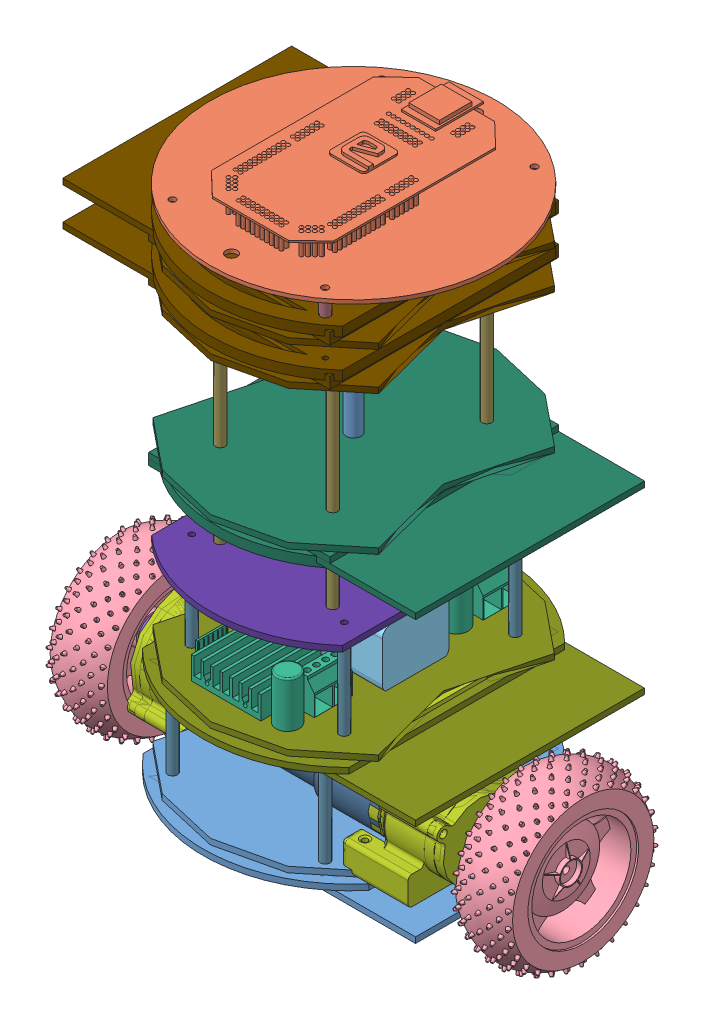
SolidWorks assembly Final_Assembly, configuration Default. Lengths in mm.
Overall size (242.54 314.31 157.59).
55 component instances, 25 part files, 122 mates.
Components (placement in the parent):
- Base_Plate-1: Base_Plate [Default] at (23.8966 49.5852 184.3209) size (151.66 9 157.59)
- eYFi_Mega-1: eYFi_Mega [Default] at (51.3966 328.5852 178.3209) size (150 18 150)
- LINE_SENSOR-1: LINE_SENSOR [Default] at (121.3966 52.5852 138.3209) x (-1 0 0) z (0 0 1) size (100 13.5 28)
- 85mm_Wheel-1: 85mm_Wheel [Default] at (-34.8424 63.1927 125.1203) x (0 0 1) z (0 -1 0) size (89.76 30.03 89.76)
- Bearing_large-1: Bearing_large [Default] at (-10.9424 63.1927 125.1203) x (0 0 1) z (-1 0 0) size (34 34 10)
- Bearing_Small-1: Bearing_Small [Default] at (10.4876 63.1927 125.1203) x (0 0 1) z (-1 0 0) size (16 16 5)
- Gear_Box_Covering - Modifiable-1: Gear_Box_Covering - Modifiable [Default] at (5.4876 63.1927 125.1203) x (0 -0.541121 0.840945) z (-1 0 0) size (87.3 57.46 46.55)
- Gear_Driven-1: Gear_Driven [Default] at (-4.4424 63.1927 125.1203) x (0 0 1) z (-1 0 0) size (41.92 41.92 47.93)
- Gear_Driver-1: Gear_Driver [Default] at (-1.5124 79.5886 99.6397) x (0 0.924225 0.381849) z (-1 0 0) size (21.81 21.81 25.3)
- IG32_MOTORS-1: IG32_MOTORS [Default] at (15.4876 79.5886 99.6397) x (1 0 0) z (0 -1 0) size (92 51.5 40)
- Motor_Main_Shaft-1: Motor_Main_Shaft [Default] at (15.4876 79.5886 99.6397) x (0 0.924225 0.381849) z (-1 0 0) size (6 6 15)
- Bearing_Small-2: Bearing_Small [Default] at (-10.9424 79.5886 99.6397) x (0 0 1) z (-1 0 0) size (16 16 5)
- Bearing_Small-3: Bearing_Small [Default] at (153.7356 79.5886 150.6022) x (0 0 -1) z (1 0 0) size (16 16 5)
- Motor_Main_Shaft-2: Motor_Main_Shaft [Default] at (127.3056 79.5886 150.6022) x (0 0.924225 -0.381849) z (1 0 0) size (6 6 15)
- Gear_Driver-2: Gear_Driver [Default] at (144.3056 79.5886 150.6022) x (0 0.924225 -0.381849) z (1 0 0) size (21.81 21.81 25.3)
- IG32_MOTORS-2: IG32_MOTORS [Default] at (127.3056 79.5886 150.6022) x (-1 0 0) z (0 -1 0) size (92 51.5 40)
- Gear_Driven-2: Gear_Driven [Default] at (147.2356 63.1927 125.1216) x (0 0 -1) z (1 0 0) size (41.92 41.92 47.93)
- Gear_Box_Covering - Modifiable-2: Gear_Box_Covering - Modifiable [Default] at (137.3056 63.1927 125.1216) x (0 -0.541121 -0.840945) z (1 0 0) size (87.3 57.46 46.55)
- Bearing_Small-4: Bearing_Small [Default] at (132.3056 63.1927 125.1216) x (0 0 -1) z (1 0 0) size (16 16 5)
- Bearing_large-2: Bearing_large [Default] at (153.7356 63.1927 125.1216) x (0 0 -1) z (1 0 0) size (34 34 10)
- 85mm_Wheel-2: 85mm_Wheel [Default] at (177.6356 63.1927 125.1216) x (0 0 -1) z (0 -1 0) size (89.76 30.03 89.76)
- 15cm_spacers-1: 15cm_spacers [Default] at (100.8966 306.5852 164.6709) x (0.33917 0 -0.940725) z (0 -1 0) size (5 5 150)
- 15cm_spacers-2: 15cm_spacers [Default] at (41.8966 306.5852 83.8709) x (-0.113141 0 -0.993579) z (0 -1 0) size (5 5 150)
- 15cm_spacers-3: 15cm_spacers [Default] at (41.8966 306.5852 164.6709) x (0.79531 0 -0.606203) z (0 -1 0) size (5 5 150)
- 15cm_spacers-4: 15cm_spacers [Default] at (100.8966 306.5852 83.8709) x (0.903566 0 -0.428448) z (0 -1 0) size (5 5 150)
- 1cm_spacers-1: 1cm_spacers [Default] at (31.3966 316.5852 179.1209) x (-0.837169 0 -0.546944) z (-0.546944 0 0.837169) size (5 10 5)
- 1cm_spacers-2: 1cm_spacers [Default] at (111.3966 316.5852 179.1209) x (-0.837169 0 -0.546944) z (-0.546944 0 0.837169) size (5 10 5)
- 1cm_spacers-3: 1cm_spacers [Default] at (111.3966 316.5852 69.4209) x (-0.837169 0 -0.546944) z (-0.546944 0 0.837169) size (5 10 5)
- 1cm_spacers-4: 1cm_spacers [Default] at (31.3966 316.5852 69.4209) x (-0.837169 0 -0.546944) z (-0.546944 0 0.837169) size (5 10 5)
- 5cm_spacers-1: 5cm_spacers [Default] at (31.3966 105.5852 69.4709) x (0.326731 0 0.945117) z (0 -1 0) size (5 5 55)
- 5cm_spacers-2: 5cm_spacers [Default] at (111.3966 105.5852 179.1709) x (1 0 0) z (0 -1 0) size (5 5 55)
- 5cm_spacers-3: 5cm_spacers [Default] at (31.3966 105.5852 179.1709) x (0.06859 0 -0.997645) z (0 -1 0) size (5 5 55)
- 5cm_spacers-4: 5cm_spacers [Default] at (111.3966 105.5852 69.4709) x (0.887621 0 0.460574) z (0 -1 0) size (5 5 55)
- 5cm_spacers-5: 5cm_spacers [Default] at (31.3966 158.5852 169.1709) x (0.326731 0 0.945117) z (0 -1 0) size (5 5 55)
- 5cm_spacers-6: 5cm_spacers [Default] at (111.3558 158.5852 169.1709) x (0.995437 0 -0.095423) z (0 -1 0) size (5 5 55)
- 5cm_spacers-7: 5cm_spacers [Default] at (111.3966 158.5852 79.4709) x (0.819559 0 -0.572995) z (0 -1 0) size (5 5 55)
- 5cm_spacers-8: 5cm_spacers [Default] at (31.3966 158.5852 79.4709) x (0.326731 0 0.945117) z (0 -1 0) size (5 5 55)
- Dead_weight-1: Dead_weight [Default] at (23.9355 196.5983 184.2695) size (151.66 12 150)
- Floor_Plates_Bottom-1: Floor_Plates_Bottom [Default] at (23.8966 102.5852 184.3209) size (151.66 9 157.59)
- Floor_Plates_Mid-1: Floor_Plates_Mid [Default] at (71.3966 158.5852 124.2709) size (100 6 150)
- Floor_Plates_Top-1: Floor_Plates_Top [Default] at (118.8966 284.5852 184.2709) x (-1 0 0) z (0 0 1) size (151.66 11 150)
- Floor_Plates_Top-2: Floor_Plates_Top [Default] at (118.8966 304.5852 184.2709) x (-1 0 0) z (0 0 1) size (151.66 11 150)
- Lead_Screw-1: Lead_Screw [Default] at (71.3966 161.5852 124.2709) size (7.8 150 7.8)
- Bearing_Small-5: Bearing_Small [Default] at (11.3966 281.5852 124.2709) x (0 0 1) z (0 1 0) size (16 16 5)
- Bearing_Small-6: Bearing_Small [Default] at (11.3966 301.5852 124.2709) x (0 0 1) z (0 1 0) size (16 16 5)
- Bearing_Small-7: Bearing_Small [Default] at (71.3966 301.5852 124.2709) x (0 0 1) z (0 1 0) size (16 16 5)
- Bearing_Small-8: Bearing_Small [Default] at (71.3966 281.5852 124.2709) x (0 0 1) z (0 1 0) size (16 16 5)
- Bearing_Small-9: Bearing_Small [Default] at (71.3966 159.5852 124.2709) x (0 0 1) z (0 1 0) size (16 16 5)
- Gear_1-1: Gear_1 [Default] at (71.3966 293.241 124.2709) x (0.999482 0 0.032177) z (0 1 0) size (64 63.73 5)
- Gear_2-1: Gear_2 [Default] at (11.3966 293.1581 124.2709) x (0.938364 0 -0.345648) z (0 -1 0) size (64 63.74 5)
- gear_shaft-1: gear_shaft [Default] at (11.3966 281.5852 124.2709) x (1 0 0) z (0 1 0) size (6 6 25)
- BATTERY-1: BATTERY [Default] at (38.4746 110.5852 106.2915) size (65 30 35)
- Motor_Driver-1: Motor_Driver [Default] at (71.3966 108.5852 80.0336) size (71 27 36.5)
- Velcro-1: Velcro [Default] at (21.3966 108.5852 144.3209) size (100 2 40)
- Motor_Driver-2: Motor_Driver [Default] at (71.3966 108.5852 168.6083) size (71 27 36.5)
Mates (geometry in assembly coordinates):
- Coincident1: coincident anti-aligned: plane of Base_Plate-1 through (142.21 52.5852 124.3209) normal (0 -1 0); plane of LINE_SENSOR-1 through (121.3966 52.5852 138.3209) normal (0 1 0)
- Concentric1: concentric anti-aligned: cylinder of Base_Plate-1 through (71.3966 60.5852 135.8209) axis (0 -1 0) radius 1.711; cylinder of LINE_SENSOR-1 through (71.3966 50.5852 135.8209) axis (0 1 0) radius 1.5
- Parallel1: parallel aligned: plane of Base_Plate-1 through (32.3966 60.5852 129.8209) normal (1 0 0); plane of LINE_SENSOR-1 through (43.3966 57.5852 128.8209) normal (1 0 0)
- Concentric2: concentric anti-aligned: cylinder of Gear_Box_Covering - Modifiable-1 through (10.4876 63.1927 125.1203) axis (-1 0 0) radius 8.75; cylinder of Gear_Driven-1 through (-33.2424 63.1927 125.1203) axis (1 0 0) radius 7.5
- Concentric3: concentric anti-aligned: cylinder of Bearing_Small-1 through (10.4876 63.1927 125.1203) axis (-1 0 0) radius 8; cylinder of Gear_Driven-1 through (-33.2424 63.1927 125.1203) axis (1 0 0) radius 7.5
- Coincident3: coincident anti-aligned: plane of Bearing_Small-1 through (10.4876 63.1927 125.1203) normal (1 0 0); plane of Gear_Box_Covering - Modifiable-1 through (10.4876 63.1927 125.1203) normal (-1 0 0)
- Coincident4: coincident anti-aligned: plane of Gear_Box_Covering - Modifiable-1 through (10.4876 63.1927 125.1203) normal (-1 0 0); plane of Gear_Driven-1 through (10.4876 63.1927 125.1203) normal (1 0 0)
- Concentric4: concentric aligned: cylinder of IG32_MOTORS-1 through (12.4876 79.5886 99.6397) axis (1 0 0) radius 7.5; cylinder of Motor_Main_Shaft-1 through (0.4876 79.5886 99.6397) axis (1 0 0) radius 3
- Coincident5: coincident anti-aligned: plane of IG32_MOTORS-1 through (15.4876 79.5886 99.6397) normal (-1 0 0); plane of Motor_Main_Shaft-1 through (15.4876 79.5886 99.6397) normal (1 0 0)
- Concentric5: concentric anti-aligned: cylinder of Gear_Driver-1 through (6.4876 84.5527 87.6247) axis (0 -0.381849 0.924225) radius 2; cylinder of Motor_Main_Shaft-1 through (6.4876 78.2522 102.8745) axis (0 0.381849 -0.924225) radius 1.5
- Concentric6: concentric anti-aligned: cylinder of Gear_Driver-1 through (12.4876 79.5886 99.6397) axis (-1 0 0) radius 5.75; cylinder of Motor_Main_Shaft-1 through (0.4876 79.5886 99.6397) axis (1 0 0) radius 3
- Parallel2: parallel aligned: plane of 85mm_Wheel-1 through (-33.2424 66.6677 131.1392) normal (0 0 -1); plane of Gear_Driven-1 through (-37.4424 66.6677 119.1014) normal (0 0 -1)
- Concentric7: concentric aligned: cylinder of 85mm_Wheel-1 through (-43.4424 63.1927 125.1203) axis (1 0 0) radius 5.5; cylinder of Gear_Driven-1 through (-33.2424 63.1927 125.1203) axis (1 0 0) radius 7.5
- Coincident7: coincident anti-aligned: plane of 85mm_Wheel-1 through (-37.4424 63.1927 125.1203) normal (1 0 0); plane of Gear_Driven-1 through (-37.4424 63.1927 125.1203) normal (-1 0 0)
- Concentric8: concentric anti-aligned: cylinder of Gear_Box_Covering - Modifiable-1 through (0.4876 79.5886 99.6397) axis (1 0 0) radius 10.75; cylinder of Bearing_Small-2 through (-10.9424 79.5886 99.6397) axis (-1 0 0) radius 8
- Coincident8: coincident aligned: plane of Gear_Box_Covering - Modifiable-1 through (-15.9424 85.9303 79.6201) normal (-1 0 0); plane of Bearing_Small-2 through (-15.9424 79.5886 99.6397) normal (-1 0 0)
- Concentric9: concentric anti-aligned: cylinder of Gear_Box_Covering - Modifiable-1 through (0.4876 79.5886 99.6397) axis (1 0 0) radius 10.75; cylinder of Gear_Driver-1 through (-2.0124 79.5886 99.6397) axis (-1 0 0) radius 2.8
- Concentric13: concentric anti-aligned: cylinder of Bearing_large-1 through (-10.9424 63.1927 125.1203) axis (-1 0 0) radius 17; cylinder of Gear_Driven-1 through (-33.2424 63.1927 125.1203) axis (1 0 0) radius 7.5
- Coincident14: coincident aligned: plane of Bearing_large-1 through (-20.9424 63.1927 125.1203) normal (-1 0 0); plane of Gear_Box_Covering - Modifiable-1 through (-20.9424 63.1927 125.1203) normal (-1 0 0)
- Parallel5: parallel anti-aligned: plane of Base_Plate-1 through (12.2366 52.5852 78.2222) normal (-1 0 0); plane of Gear_Box_Covering - Modifiable-1 through (25.4876 63.1927 125.1203) normal (1 0 0)
- Parallel6: parallel anti-aligned: plane of Base_Plate-1 through (142.21 55.5852 124.3209) normal (0 1 0); plane of Gear_Box_Covering - Modifiable-1 through (25.4876 55.5852 125.1203) normal (0 -1 0)
- Concentric14: concentric aligned: cylinder of Base_Plate-1 through (18.7376 44.5852 79.3183) axis (0 1 0) radius 1.75; cylinder of Gear_Box_Covering - Modifiable-1 through (18.7376 45.4192 79.3183) axis (0 1 0) radius 1.5
- Coincident18: coincident anti-aligned: plane of Base_Plate-1 through (142.21 55.5852 124.3209) normal (0 1 0); plane of Gear_Box_Covering - Modifiable-1 through (25.4876 55.5852 125.1203) normal (0 -1 0)
- Concentric16: concentric aligned: cylinder of Gear_Box_Covering - Modifiable-1 through (10.4876 93.0886 99.6397) axis (-1 0 0) radius 1.75; cylinder of IG32_MOTORS-1 through (18.4876 93.0886 99.6397) axis (-1 0 0) radius 1.5
- Coincident19: coincident anti-aligned: plane of Gear_Box_Covering - Modifiable-1 through (15.4876 79.5886 99.6397) normal (1 0 0); plane of IG32_MOTORS-1 through (15.4876 79.5886 99.6397) normal (-1 0 0)
- Concentric17: concentric aligned: cylinder of IG32_MOTORS-2 through (124.3056 93.0886 150.6022) axis (1 0 0) radius 1.5; cylinder of Gear_Box_Covering - Modifiable-2 through (132.3056 93.0886 150.6022) axis (1 0 0) radius 1.75
- Coincident20: coincident aligned: plane of Gear_Box_Covering - Modifiable-2 through (163.7356 63.1927 125.1216) normal (1 0 0); plane of Bearing_large-2 through (163.7356 63.1927 125.1216) normal (1 0 0)
- Coincident21: coincident aligned: plane of Bearing_Small-3 through (158.7356 79.5886 150.6022) normal (1 0 0); plane of Gear_Box_Covering - Modifiable-2 through (158.7356 85.9303 170.6218) normal (1 0 0)
- Coincident22: coincident anti-aligned: plane of Motor_Main_Shaft-2 through (127.3056 79.5886 150.6022) normal (-1 0 0); plane of IG32_MOTORS-2 through (127.3056 79.5886 150.6022) normal (1 0 0)
- Parallel7: parallel aligned: plane of Gear_Driven-2 through (180.2356 66.6677 131.1405) normal (0 0 1); plane of 85mm_Wheel-2 through (176.0356 66.6677 119.1027) normal (0 0 1)
- Coincident23: coincident anti-aligned: plane of Gear_Driven-2 through (132.3056 63.1927 125.1216) normal (-1 0 0); plane of Gear_Box_Covering - Modifiable-2 through (132.3056 63.1927 125.1216) normal (1 0 0)
- Coincident24: coincident anti-aligned: plane of Gear_Box_Covering - Modifiable-2 through (132.3056 63.1927 125.1216) normal (1 0 0); plane of Bearing_Small-4 through (132.3056 63.1927 125.1216) normal (-1 0 0)
- Coincident25: coincident anti-aligned: plane of Gear_Driven-2 through (180.2356 63.1927 125.1216) normal (1 0 0); plane of 85mm_Wheel-2 through (180.2356 63.1927 125.1216) normal (-1 0 0)
- Concentric18: concentric anti-aligned: cylinder of Gear_Driven-2 through (176.0356 63.1927 125.1216) axis (-1 0 0) radius 7.5; cylinder of Gear_Box_Covering - Modifiable-2 through (132.3056 63.1927 125.1216) axis (1 0 0) radius 8.75
- Concentric19: concentric anti-aligned: cylinder of Gear_Driven-2 through (176.0356 63.1927 125.1216) axis (-1 0 0) radius 7.5; cylinder of Bearing_large-2 through (153.7356 63.1927 125.1216) axis (1 0 0) radius 17
- Concentric20: concentric anti-aligned: cylinder of Motor_Main_Shaft-2 through (136.3056 78.2522 147.3674) axis (0 0.381849 0.924225) radius 1.5; cylinder of Gear_Driver-2 through (136.3056 84.5527 162.6171) axis (0 -0.381849 -0.924225) radius 2
- Concentric21: concentric anti-aligned: cylinder of Bearing_Small-3 through (153.7356 79.5886 150.6022) axis (1 0 0) radius 8; cylinder of Gear_Box_Covering - Modifiable-2 through (142.3056 79.5886 150.6022) axis (-1 0 0) radius 10.75
- Concentric22: concentric anti-aligned: cylinder of Gear_Driven-2 through (176.0356 63.1927 125.1216) axis (-1 0 0) radius 7.5; cylinder of Bearing_Small-4 through (132.3056 63.1927 125.1216) axis (1 0 0) radius 8
- Concentric23: concentric anti-aligned: cylinder of Gear_Driver-2 through (144.8056 79.5886 150.6022) axis (1 0 0) radius 2.8; cylinder of Gear_Box_Covering - Modifiable-2 through (142.3056 79.5886 150.6022) axis (-1 0 0) radius 10.75
- Concentric24: concentric aligned: cylinder of Motor_Main_Shaft-2 through (142.3056 79.5886 150.6022) axis (-1 0 0) radius 3; cylinder of IG32_MOTORS-2 through (130.3056 79.5886 150.6022) axis (-1 0 0) radius 7.5
- Concentric25: concentric anti-aligned: cylinder of Motor_Main_Shaft-2 through (142.3056 79.5886 150.6022) axis (-1 0 0) radius 3; cylinder of Gear_Driver-2 through (130.3056 79.5886 150.6022) axis (1 0 0) radius 5.75
- Concentric26: concentric aligned: cylinder of Gear_Driven-2 through (176.0356 63.1927 125.1216) axis (-1 0 0) radius 7.5; cylinder of 85mm_Wheel-2 through (186.2356 63.1927 125.1216) axis (-1 0 0) radius 5.5
- Coincident26: coincident anti-aligned: plane of IG32_MOTORS-2 through (127.3056 79.5886 150.6022) normal (1 0 0); plane of Gear_Box_Covering - Modifiable-2 through (127.3056 79.5886 150.6022) normal (-1 0 0)
- Concentric27: concentric aligned: cylinder of Base_Plate-1 through (124.0556 44.5852 170.9235) axis (0 1 0) radius 1.75; cylinder of Gear_Box_Covering - Modifiable-2 through (124.0556 45.4192 170.9235) axis (0 1 0) radius 1.5
- Coincident27: coincident anti-aligned: plane of Base_Plate-1 through (142.21 55.5852 124.3209) normal (0 1 0); plane of Gear_Box_Covering - Modifiable-2 through (117.3056 55.5852 125.1216) normal (0 -1 0)
- Parallel8: parallel anti-aligned: plane of Base_Plate-1 through (130.5566 52.5852 78.2222) normal (1 0 0); plane of Gear_Box_Covering - Modifiable-2 through (117.3056 63.1927 125.1216) normal (-1 0 0)
- Concentric28: concentric anti-aligned: cylinder of Base_Plate-1 through (31.3966 62.5852 179.1709) axis (0 -1 0) radius 1.25; cylinder of 5cm_spacers-3 through (31.3966 50.5852 179.1709) axis (0 1 0) radius 1.25
- Concentric29: concentric anti-aligned: cylinder of Base_Plate-1 through (111.3966 62.5852 179.1709) axis (0 -1 0) radius 1.25; cylinder of 5cm_spacers-2 through (111.3966 55.5852 179.1709) axis (0 1 0) radius 2.5
- Concentric30: concentric anti-aligned: cylinder of Base_Plate-1 through (111.3966 62.5852 69.4709) axis (0 -1 0) radius 1.25; cylinder of 5cm_spacers-4 through (111.3966 50.5852 69.4709) axis (0 1 0) radius 1.25
- Concentric31: concentric anti-aligned: cylinder of Base_Plate-1 through (31.3966 62.5852 69.4709) axis (0 -1 0) radius 1.25; cylinder of 5cm_spacers-1 through (31.3966 55.5852 69.4709) axis (0 1 0) radius 2.5
- Coincident28: coincident anti-aligned: plane of Base_Plate-1 through (142.21 55.5852 124.3209) normal (0 1 0); plane of 5cm_spacers-3 through (31.3966 55.5852 179.1709) normal (0 -1 0)
- Coincident29: coincident anti-aligned: plane of Base_Plate-1 through (142.21 55.5852 124.3209) normal (0 1 0); plane of 5cm_spacers-2 through (111.3966 55.5852 179.1709) normal (0 -1 0)
- Coincident30: coincident anti-aligned: plane of Base_Plate-1 through (142.21 55.5852 124.3209) normal (0 1 0); plane of 5cm_spacers-4 through (111.3966 55.5852 69.4709) normal (0 -1 0)
- Coincident31: coincident anti-aligned: plane of Base_Plate-1 through (142.21 55.5852 124.3209) normal (0 1 0); plane of 5cm_spacers-1 through (31.3966 55.5852 69.4709) normal (0 -1 0)
- Concentric32: concentric anti-aligned: cylinder of 5cm_spacers-1 through (31.3966 55.5852 69.4709) axis (0 1 0) radius 2.5; cylinder of Floor_Plates_Bottom-1 through (31.3966 115.5852 69.4709) axis (0 -1 0) radius 1.25
- Concentric33: concentric anti-aligned: cylinder of 5cm_spacers-4 through (111.3966 55.5852 69.4709) axis (0 1 0) radius 2.5; cylinder of Floor_Plates_Bottom-1 through (111.3966 115.5852 69.4709) axis (0 -1 0) radius 1.25
- Coincident32: coincident anti-aligned: plane of 5cm_spacers-4 through (111.3966 105.5852 69.4709) normal (0 1 0); plane of Floor_Plates_Bottom-1 through (142.21 105.5852 124.3209) normal (0 -1 0)
- Concentric34: concentric anti-aligned: cylinder of 5cm_spacers-5 through (31.3966 103.5852 169.1709) axis (0 1 0) radius 1.25; cylinder of Floor_Plates_Bottom-1 through (31.3966 115.5852 169.1709) axis (0 -1 0) radius 1.5
- Concentric35: concentric anti-aligned: cylinder of 5cm_spacers-6 through (111.3558 108.5852 169.1709) axis (0 1 0) radius 2.5; cylinder of Floor_Plates_Bottom-1 through (111.3558 115.5852 169.1709) axis (0 -1 0) radius 1.5
- Concentric36: concentric anti-aligned: cylinder of 5cm_spacers-7 through (111.3966 108.5852 79.4709) axis (0 1 0) radius 2.5; cylinder of Floor_Plates_Bottom-1 through (111.3966 115.5852 79.4709) axis (0 -1 0) radius 1.5
- Concentric37: concentric anti-aligned: cylinder of 5cm_spacers-8 through (31.3966 108.5852 79.4709) axis (0 1 0) radius 2.5; cylinder of Floor_Plates_Bottom-1 through (31.3966 115.5852 79.4709) axis (0 -1 0) radius 1.5
- Coincident33: coincident anti-aligned: plane of 5cm_spacers-8 through (31.3966 108.5852 79.4709) normal (0 -1 0); plane of Floor_Plates_Bottom-1 through (142.21 108.5852 124.3209) normal (0 1 0)
- Coincident35: coincident anti-aligned: plane of 5cm_spacers-7 through (111.3966 108.5852 79.4709) normal (0 -1 0); plane of Floor_Plates_Bottom-1 through (142.21 108.5852 124.3209) normal (0 1 0)
- Coincident36: coincident anti-aligned: plane of 5cm_spacers-5 through (31.3966 108.5852 169.1709) normal (0 -1 0); plane of Floor_Plates_Bottom-1 through (142.21 108.5852 124.3209) normal (0 1 0)
- Coincident37: coincident anti-aligned: plane of 5cm_spacers-6 through (111.3558 108.5852 169.1709) normal (0 -1 0); plane of Floor_Plates_Bottom-1 through (142.21 108.5852 124.3209) normal (0 1 0)
- Concentric38: concentric anti-aligned: cylinder of 5cm_spacers-5 through (31.3966 108.5852 169.1709) axis (0 1 0) radius 2.5; cylinder of Floor_Plates_Mid-1 through (31.3966 161.5852 169.1709) axis (0 -1 0) radius 1.5
- Coincident39: coincident anti-aligned: plane of 5cm_spacers-6 through (111.3558 158.5852 169.1709) normal (0 1 0); plane of Floor_Plates_Mid-1 through (71.3966 158.5852 124.2709) normal (0 -1 0)
- Parallel11: parallel aligned: plane of Floor_Plates_Bottom-1 through (125.5556 115.5852 184.3209) normal (1 0 0); plane of Floor_Plates_Mid-1 through (121.3966 161.5852 124.2709) normal (1 0 0)
- Concentric41: concentric anti-aligned: cylinder of 15cm_spacers-3 through (41.8966 161.5852 164.6709) axis (0 1 0) radius 2.5; cylinder of Floor_Plates_Mid-1 through (41.8966 161.5852 164.6709) axis (0 -1 0) radius 1.5
- Concentric42: concentric anti-aligned: cylinder of 15cm_spacers-1 through (100.8966 161.5852 164.6709) axis (0 1 0) radius 2.5; cylinder of Floor_Plates_Mid-1 through (100.8966 161.5852 164.6709) axis (0 -1 0) radius 1.5
- Concentric43: concentric anti-aligned: cylinder of 15cm_spacers-2 through (41.8966 161.5852 83.8709) axis (0 1 0) radius 2.5; cylinder of Floor_Plates_Mid-1 through (41.8966 161.5852 83.8709) axis (0 -1 0) radius 1.5
- Concentric44: concentric anti-aligned: cylinder of 15cm_spacers-4 through (100.8966 161.5852 83.8709) axis (0 1 0) radius 2.5; cylinder of Floor_Plates_Mid-1 through (100.8966 161.5852 83.8709) axis (0 -1 0) radius 1.5
- Coincident42: coincident anti-aligned: plane of 15cm_spacers-4 through (100.8966 161.5852 83.8709) normal (0 -1 0); plane of Floor_Plates_Mid-1 through (71.3966 161.5852 124.2709) normal (0 1 0)
- Coincident43: coincident anti-aligned: plane of 15cm_spacers-1 through (100.8966 161.5852 164.6709) normal (0 -1 0); plane of Floor_Plates_Mid-1 through (71.3966 161.5852 124.2709) normal (0 1 0)
- Coincident44: coincident anti-aligned: plane of 15cm_spacers-3 through (41.8966 161.5852 164.6709) normal (0 -1 0); plane of Floor_Plates_Mid-1 through (71.3966 161.5852 124.2709) normal (0 1 0)
- Coincident45: coincident anti-aligned: plane of 15cm_spacers-2 through (41.8966 161.5852 83.8709) normal (0 -1 0); plane of Floor_Plates_Mid-1 through (71.3966 161.5852 124.2709) normal (0 1 0)
- Concentric45: concentric aligned: cylinder of Floor_Plates_Top-1 through (71.3966 286.5852 124.2709) axis (0 -1 0) radius 75; cylinder of Floor_Plates_Top-2 through (71.3966 306.5852 124.2709) axis (0 -1 0) radius 75
- Parallel12: parallel aligned: plane of Floor_Plates_Mid-1 through (121.3966 161.5852 124.2709) normal (1 0 0); plane of Floor_Plates_Top-1 through (121.3966 291.5852 184.2709) normal (1 0 0)
- Concentric46: concentric aligned: cylinder of Floor_Plates_Mid-1 through (71.3966 164.5852 124.2709) axis (0 -1 0) radius 8.35; cylinder of Floor_Plates_Top-1 through (71.3966 291.5852 124.2709) axis (0 -1 0) radius 8.4
- Coincident47: coincident aligned: plane of 15cm_spacers-3 through (41.8966 306.5852 164.6709) normal (0 1 0); plane of Floor_Plates_Top-2 through (71.3966 306.5852 124.2709) normal (0 1 0)
- Concentric47: concentric anti-aligned: cylinder of 15cm_spacers-4 through (100.8966 161.5852 83.8709) axis (0 1 0) radius 2.5; cylinder of Dead_weight-1 through (100.8966 206.5983 83.8709) axis (0 -1 0) radius 3.5
- Parallel13: parallel aligned: plane of Dead_weight-1 through (126.4355 204.5983 184.2695) normal (1 0 0); plane of Floor_Plates_Bottom-1 through (125.5556 115.5852 184.3209) normal (1 0 0)
- Concentric48: concentric aligned: cylinder of 1cm_spacers-1 through (31.3966 306.5852 179.1209) axis (0 1 0) radius 2.5; cylinder of Floor_Plates_Top-2 through (31.3966 291.5852 179.1209) axis (0 1 0) radius 1.25
- Concentric49: concentric aligned: cylinder of 1cm_spacers-2 through (111.3966 306.5852 179.1209) axis (0 1 0) radius 2.5; cylinder of Floor_Plates_Top-2 through (111.3966 291.5852 179.1209) axis (0 1 0) radius 1.25
- Concentric50: concentric aligned: cylinder of 1cm_spacers-3 through (111.3966 306.5852 69.4209) axis (0 1 0) radius 2.5; cylinder of Floor_Plates_Top-2 through (111.3966 291.5852 69.4209) axis (0 1 0) radius 1.25
- Concentric52: concentric aligned: cylinder of 1cm_spacers-4 through (31.3966 306.5852 69.4209) axis (0 1 0) radius 2.5; cylinder of Floor_Plates_Top-2 through (31.3966 291.5852 69.4209) axis (0 1 0) radius 1.25
- Coincident49: coincident anti-aligned: plane of 1cm_spacers-2 through (111.3966 306.5852 179.1209) normal (0 -1 0); plane of Floor_Plates_Top-2 through (71.3966 306.5852 124.2709) normal (0 1 0)
- Coincident51: coincident anti-aligned: plane of 1cm_spacers-1 through (31.3966 306.5852 179.1209) normal (0 -1 0); plane of Floor_Plates_Top-2 through (71.3966 306.5852 124.2709) normal (0 1 0)
- Coincident52: coincident anti-aligned: plane of 1cm_spacers-4 through (31.3966 306.5852 69.4209) normal (0 -1 0); plane of Floor_Plates_Top-2 through (71.3966 306.5852 124.2709) normal (0 1 0)
- Coincident53: coincident anti-aligned: plane of 1cm_spacers-3 through (111.3966 306.5852 69.4209) normal (0 -1 0); plane of Floor_Plates_Top-2 through (71.3966 306.5852 124.2709) normal (0 1 0)
- Concentric53: concentric aligned: cylinder of Floor_Plates_Mid-1 through (71.3966 164.5852 124.2709) axis (0 -1 0) radius 8.35; cylinder of Lead_Screw-1 through (71.3966 311.5852 124.2709) axis (0 -1 0) radius 3.9
- Coincident54: coincident anti-aligned: plane of Floor_Plates_Mid-1 through (71.3966 161.5852 124.2709) normal (0 1 0); plane of Lead_Screw-1 through (71.3966 161.5852 124.2709) normal (0 -1 0)
- Concentric54: concentric anti-aligned: cylinder of Floor_Plates_Mid-1 through (71.3966 164.5852 124.2709) axis (0 -1 0) radius 8.35; cylinder of Bearing_Small-9 through (71.3966 159.5852 124.2709) axis (0 1 0) radius 8
- Coincident55: coincident aligned: plane of Floor_Plates_Mid-1 through (71.3966 164.5852 124.2709) normal (0 1 0); plane of Bearing_Small-9 through (71.3966 164.5852 124.2709) normal (0 1 0)
- Concentric55: concentric anti-aligned: cylinder of Floor_Plates_Top-2 through (11.3966 311.5852 124.2709) axis (0 -1 0) radius 8.4; cylinder of Bearing_Small-5 through (11.3966 281.5852 124.2709) axis (0 1 0) radius 8
- Concentric56: concentric anti-aligned: cylinder of Floor_Plates_Top-2 through (11.3966 311.5852 124.2709) axis (0 -1 0) radius 8.4; cylinder of Bearing_Small-6 through (11.3966 301.5852 124.2709) axis (0 1 0) radius 8
- Coincident56: coincident aligned: plane of Floor_Plates_Top-2 through (71.3966 306.5852 124.2709) normal (0 1 0); plane of Bearing_Small-6 through (11.3966 306.5852 124.2709) normal (0 1 0)
- Coincident57: coincident aligned: plane of Floor_Plates_Top-1 through (71.3966 286.5852 124.2709) normal (0 1 0); plane of Bearing_Small-5 through (11.3966 286.5852 124.2709) normal (0 1 0)
- Concentric57: concentric anti-aligned: cylinder of Lead_Screw-1 through (71.3966 311.5852 124.2709) axis (0 -1 0) radius 3.9; cylinder of Bearing_Small-7 through (71.3966 301.5852 124.2709) axis (0 1 0) radius 8
- Coincident58: coincident aligned: plane of Floor_Plates_Top-2 through (71.3966 306.5852 124.2709) normal (0 1 0); plane of Bearing_Small-7 through (71.3966 306.5852 124.2709) normal (0 1 0)
- Concentric58: concentric anti-aligned: cylinder of Floor_Plates_Top-1 through (71.3966 291.5852 124.2709) axis (0 -1 0) radius 8.4; cylinder of Bearing_Small-8 through (71.3966 281.5852 124.2709) axis (0 1 0) radius 8
- Coincident59: coincident aligned: plane of Floor_Plates_Top-1 through (71.3966 281.5852 124.2709) normal (0 -1 0); plane of Bearing_Small-8 through (71.3966 281.5852 124.2709) normal (0 -1 0)
- Concentric59: concentric aligned: cylinder of 1cm_spacers-3 through (111.3966 306.5852 69.4209) axis (0 1 0) radius 2.5; cylinder of eYFi_Mega-1 through (111.3966 308.5852 69.4209) axis (0 1 0) radius 1.75
- Concentric60: concentric aligned: cylinder of 1cm_spacers-4 through (31.3966 306.5852 69.4209) axis (0 1 0) radius 2.5; cylinder of eYFi_Mega-1 through (31.3966 308.5852 69.4209) axis (0 1 0) radius 1.75
- Coincident60: coincident anti-aligned: plane of 1cm_spacers-4 through (31.3966 316.5852 69.4209) normal (0 1 0); plane of eYFi_Mega-1 through (71.3966 316.5852 124.3209) normal (0 -1 0)
- Parallel14: parallel aligned: plane of Floor_Plates_Top-1 through (121.3966 291.5852 184.2709) normal (1 0 0); plane of Floor_Plates_Top-2 through (121.3966 311.5852 184.2709) normal (1 0 0)
- Concentric61: concentric anti-aligned: cylinder of Lead_Screw-1 through (71.3966 311.5852 124.2709) axis (0 -1 0) radius 3.9; cylinder of Gear_1-1 through (71.3966 290.741 124.2709) axis (0 1 0) radius 27.5
- Concentric63: concentric anti-aligned: cylinder of Bearing_Small-5 through (11.3966 286.5852 124.2709) axis (0 -1 0) radius 3; cylinder of Gear_2-1 through (11.3966 245.6581 124.2709) axis (0 1 0) radius 2.8
- Concentric64: concentric anti-aligned: cylinder of Gear_2-1 through (11.3966 245.6581 124.2709) axis (0 1 0) radius 2.8; cylinder of gear_shaft-1 through (11.3966 306.5852 124.2709) axis (0 -1 0) radius 3
- Coincident63: coincident aligned: plane of Floor_Plates_Top-1 through (71.3966 281.5852 124.2709) normal (0 -1 0); plane of gear_shaft-1 through (11.3966 281.5852 124.2709) normal (0 -1 0)
- Coincident64: coincident aligned: plane of Floor_Plates_Top-2 through (71.3966 306.5852 124.2709) normal (0 1 0); plane of gear_shaft-1 through (11.3966 306.5852 124.2709) normal (0 1 0)
- Concentric65: concentric anti-aligned: cylinder of Floor_Plates_Bottom-1 through (101.3966 98.5852 114.3209) axis (0 1 0) radius 1.5; cylinder of Velcro-1 through (101.3966 110.5852 114.3209) axis (0 -1 0) radius 1.5
- Concentric66: concentric anti-aligned: cylinder of Floor_Plates_Bottom-1 through (101.3966 98.5852 134.3209) axis (0 1 0) radius 1.5; cylinder of Velcro-1 through (101.3966 110.5852 134.3209) axis (0 -1 0) radius 1.5
- Coincident65: coincident anti-aligned: plane of Floor_Plates_Bottom-1 through (142.21 108.5852 124.3209) normal (0 1 0); plane of Velcro-1 through (21.3966 108.5852 144.3209) normal (0 -1 0)
- Coincident66: coincident anti-aligned: plane of BATTERY-1 through (103.4746 110.5852 141.2915) normal (0 -1 0); plane of Velcro-1 through (21.3966 110.5852 144.3209) normal (0 1 0)
- Parallel15: parallel aligned: plane of BATTERY-1 through (38.4746 110.5852 141.2915) normal (0 0 1); plane of Velcro-1 through (21.3966 110.5852 144.3209) normal (0 0 1)
- Concentric67: concentric anti-aligned: cylinder of Floor_Plates_Bottom-1 through (103.8966 115.5852 183.8583) axis (0 -1 0) radius 1.5; cylinder of Motor_Driver-2 through (103.8966 108.5852 183.8583) axis (0 1 0) radius 1.5
- Concentric68: concentric anti-aligned: cylinder of Floor_Plates_Bottom-1 through (103.8966 115.5852 153.3583) axis (0 -1 0) radius 1.5; cylinder of Motor_Driver-2 through (103.8966 108.5852 153.3583) axis (0 1 0) radius 1.5
- Coincident68: coincident anti-aligned: plane of Floor_Plates_Bottom-1 through (142.21 108.5852 124.3209) normal (0 1 0); plane of Motor_Driver-2 through (71.3966 108.5852 168.6083) normal (0 -1 0)
- Concentric69: concentric anti-aligned: cylinder of Floor_Plates_Bottom-1 through (103.8966 115.5852 95.2836) axis (0 -1 0) radius 1.5; cylinder of Motor_Driver-1 through (103.8966 108.5852 95.2836) axis (0 1 0) radius 1.5
- Concentric70: concentric anti-aligned: cylinder of Floor_Plates_Bottom-1 through (103.8966 115.5852 64.7836) axis (0 -1 0) radius 1.5; cylinder of Motor_Driver-1 through (103.8966 108.5852 64.7836) axis (0 1 0) radius 1.5
- Coincident69: coincident anti-aligned: plane of Floor_Plates_Bottom-1 through (142.21 108.5852 124.3209) normal (0 1 0); plane of Motor_Driver-1 through (71.3966 108.5852 80.0336) normal (0 -1 0)
